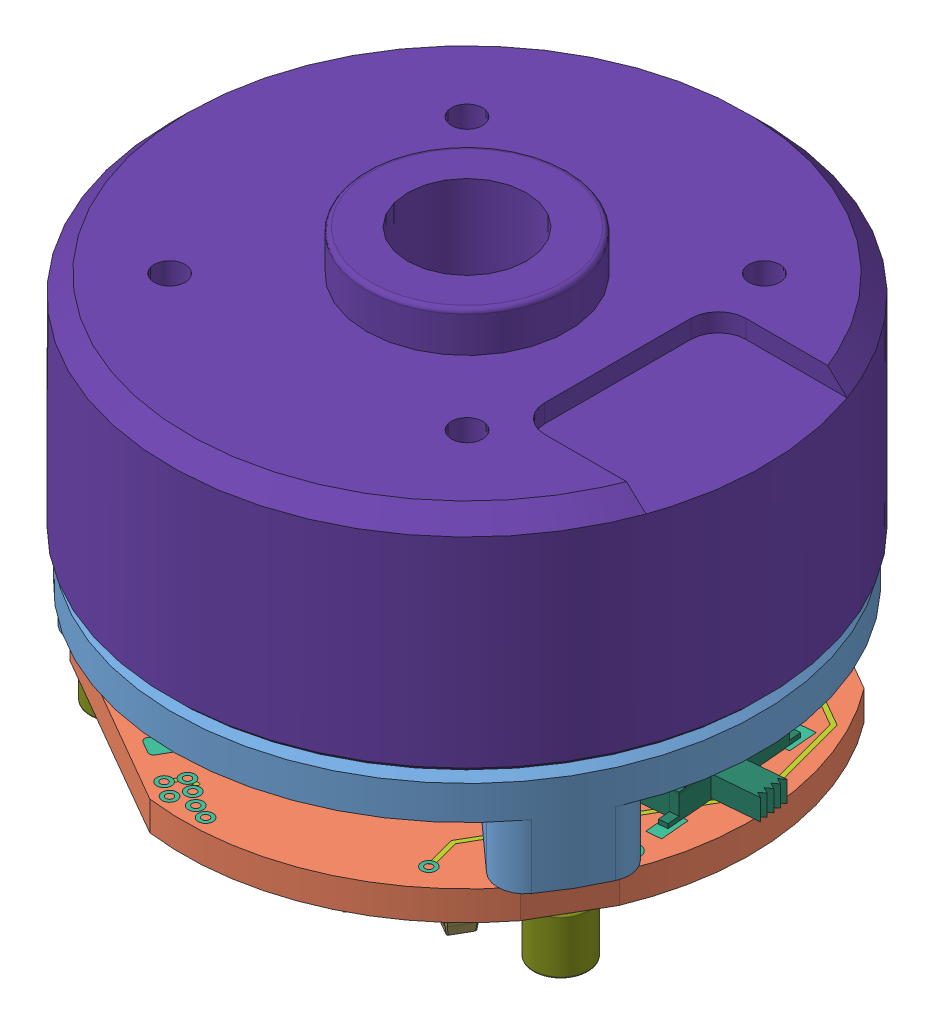
SolidWorks assembly 2804-特价电机 - 孔位修正版-减厚, configuration 默认. Lengths in mm.
Overall size (40.92 25 40.14).
94 component instances, 53 part files, 8 mates.
Components (placement in the parent):
- 复件 零件1^2804-特价电机 - 孔位修正版-减厚-1: 复件 零件1^2804-特价电机 - 孔位修正版-减厚 [默认] x (0 0 -1) z (1 0 0) size (32 6.17 30.88) (virtual)
- S28P12-1: S28P12 [默认] at (0.0001 -7.6 0.0003) x (0.5 0 -0.866025) z (0 -1 0) size (28.6 30.74 6.15)
  - S28P12.step-1: S28P12.step [默认] at origin size (28.6 30.74 6.15)
    - Board_Geoms_db26.step-1: Board_Geoms_db26.step [默认] at origin size (28.6 30.74 1.88)
      - Pcb_db26.step-1: Pcb_db26.step [默认] at (-99.9998 99.9998 0) size (28.6 30.74 1.6)
      - topPads_db26.step-1: topPads_db26.step [默认] at (-99.9998 99.9998 0.02) size (27.56 29.1 0.01)
      - topTracks_db26.step-1: topTracks_db26.step [默认] at (-99.9998 99.9998 0.01) size (26.54 27.25 0.49)
      - topZones_db26.step-1: topZones_db26.step [默认] at (-99.9998 99.9998 0.01) size (16.88 29.66 0.02)
      - botPads_db26.step-1: botPads_db26.step [默认] at (-99.9998 99.9998 -1.62) size (27.7 29.1 0.01)
      - botTracks_db26.step-1: botTracks_db26.step [默认] at (-99.9998 99.9998 -1.61) size (26.06 27.6 0.02)
      - botZones_db26.step-1: botZones_db26.step [默认] at (-99.9998 99.9998 -1.61) size (24.07 13.81 0.01)
    - Step_Models_db26.step-1: Step_Models_db26.step [默认] at origin size (26.96 28.57 6.15)
      - Top_db26.step-1: Top_db26.step [默认] at origin size (24.86 27.45 1.59)
        - U4_PWP059_00006012a0b9.step-1: U4_PWP059_00006012a0b9.step [默认] at (-0.0198 -8.0402 0) x (0 1 0) z (1 0 0) size (6.4 1.2 9.7)
          - PWP28.step-1: PWP28.step [默认] at origin size (1 0.75 0.24)
          - PWP029.step-1: PWP029.step [默认] at origin size (1 0.75 0.24)
          - PWP030.step-1: PWP030.step [默认] at origin size (1 0.75 0.24)
          - PWP031.step-1: PWP031.step [默认] at origin size (1 0.75 0.24)
          - PWP032.step-1: PWP032.step [默认] at origin size (1 0.75 0.24)
          - PWP033.step-1: PWP033.step [默认] at origin size (1 0.75 0.24)
          - PWP034.step-1: PWP034.step [默认] at origin size (1 0.75 0.24)
          - PWP035.step-1: PWP035.step [默认] at origin size (1 0.75 0.24)
          - PWP036.step-1: PWP036.step [默认] at origin size (1 0.75 0.24)
          - PWP037.step-1: PWP037.step [默认] at origin size (1 0.75 0.24)
          - PWP038.step-1: PWP038.step [默认] at origin size (1 0.75 0.24)
          - PWP039.step-1: PWP039.step [默认] at origin size (1 0.75 0.24)
          - PWP040.step-1: PWP040.step [默认] at origin size (1 0.75 0.24)
          - PWP041.step-1: PWP041.step [默认] at origin size (1 0.75 0.24)
          - PWP042.step-1: PWP042.step [默认] at origin size (1 0.75 0.24)
          - PWP043.step-1: PWP043.step [默认] at origin size (1 0.75 0.24)
          - PWP044.step-1: PWP044.step [默认] at origin size (1 0.75 0.24)
          - PWP045.step-1: PWP045.step [默认] at origin size (1 0.75 0.24)
          - PWP046.step-1: PWP046.step [默认] at origin size (1 0.75 0.24)
          - PWP047.step-1: PWP047.step [默认] at origin size (1 0.75 0.24)
          - PWP048.step-1: PWP048.step [默认] at origin size (1 0.75 0.24)
          - PWP049.step-1: PWP049.step [默认] at origin size (1 0.75 0.24)
          - PWP050.step-1: PWP050.step [默认] at origin size (1 0.75 0.24)
          - PWP051.step-1: PWP051.step [默认] at origin size (1 0.75 0.24)
          - PWP052.step-1: PWP052.step [默认] at origin size (1 0.75 0.24)
          - PWP053.step-1: PWP053.step [默认] at origin size (1 0.75 0.24)
          - PWP054.step-1: PWP054.step [默认] at origin size (1 0.75 0.24)
          - PWP055.step-1: PWP055.step [默认] at origin size (1 0.75 0.24)
          - PWP056.step-1: PWP056.step [默认] at origin size (0.55 0.05 0.55)
          - PWP057.step-1: PWP057.step [默认] at origin size (4.4 1.06 9.7)
          - PWP058.step-1: PWP058.step [默认] at origin size (2.75 0.25 5.23)
        - C2_C_0603_1608Metric_00006005682b.step-1: C2_C_0603_1608Metric_00006005682b.step [默认] at (-4.7929 -0.2178 0) x (0 1 0) z (0 0 1) size (1.6 0.8 0.8)
        - C2_C_0603_1608Metric_00006005682b.step-2: C2_C_0603_1608Metric_00006005682b.step [默认] at (-6.2929 -0.2378 0) x (0 1 0) z (0 0 1) size (1.6 0.8 0.8)
        - C2_C_0603_1608Metric_00006005682b.step-3: C2_C_0603_1608Metric_00006005682b.step [默认] at (-5.9698 -10.4127 0) x (0 -1 0) z (0 0 1) size (1.6 0.8 0.8)
        - C2_C_0603_1608Metric_00006005682b.step-4: C2_C_0603_1608Metric_00006005682b.step [默认] at (-9.9829 6.3622 0) x (0 1 0) z (0 0 1) size (1.6 0.8 0.8)
        - C2_C_0603_1608Metric_00006005682b.step-5: C2_C_0603_1608Metric_00006005682b.step [默认] at (7.5102 -10.7002 0) x (0 1 0) z (0 0 1) size (1.6 0.8 0.8)
        - C2_C_0603_1608Metric_00006005682b.step-6: C2_C_0603_1608Metric_00006005682b.step [默认] at (-2.0229 9.3422 0) x (0 1 0) z (0 0 1) size (1.6 0.8 0.8)
        - C2_C_0603_1608Metric_00006005682b.step-7: C2_C_0603_1608Metric_00006005682b.step [默认] at (-5.2298 -13.0102 0) size (1.6 0.8 0.8)
        - C2_C_0603_1608Metric_00006005682b.step-8: C2_C_0603_1608Metric_00006005682b.step [默认] at (-7.4598 -10.4002 0) x (0 1 0) z (0 0 1) size (1.6 0.8 0.8)
        - C2_C_0603_1608Metric_00006005682b.step-9: C2_C_0603_1608Metric_00006005682b.step [默认] at (7.5302 -7.6827 0) x (0 -1 0) z (0 0 1) size (1.6 0.8 0.8)
        - D2_LED_0603_1608Metric_0000600568f0.step-1: D2_LED_0603_1608Metric_0000600568f0.step [默认] at (9.0171 -7.6853 0) x (0 1 0) z (0 0 1) size (1.6 0.8 1.1)
        - R1_R_0603_1608Metric_00006005698f.step-1: R1_R_0603_1608Metric_00006005698f.step [默认] at (10.6096 8.0922 0) x (-1 0 0) z (0 0 1) size (1.6 0.8 0.45)
        - R1_R_0603_1608Metric_00006005698f.step-2: R1_R_0603_1608Metric_00006005698f.step [默认] at (9.2771 -4.0278 0) x (0 1 0) z (0 0 1) size (1.6 0.8 0.45)
        - R1_R_0603_1608Metric_00006005698f.step-3: R1_R_0603_1608Metric_00006005698f.step [默认] at (-3.3129 -1.3653 0) x (0 -1 0) z (0 0 1) size (1.6 0.8 0.45)
        - R1_R_0603_1608Metric_00006005698f.step-4: R1_R_0603_1608Metric_00006005698f.step [默认] at (0.9171 9.3297 0) x (0 1 0) z (0 0 1) size (1.6 0.8 0.45)
        - R1_R_0603_1608Metric_00006005698f.step-5: R1_R_0603_1608Metric_00006005698f.step [默认] at (-1.8229 -1.3653 0) x (0 -1 0) z (0 0 1) size (1.6 0.8 0.45)
        - R1_R_0603_1608Metric_00006005698f.step-6: R1_R_0603_1608Metric_00006005698f.step [默认] at (6.0402 -7.6827 0) x (0 -1 0) z (0 0 1) size (1.6 0.8 0.45)
        - SW1_SW_SPST_B3U-1000P_000060056a0b.step-1: SW1_SW_SPST_B3U-1000P_000060056a0b.step [默认] at (4.6571 9.5022 0) size (4 2.51 1.59)
        - U3_SOT_89_3_000060056a8b.step-1: U3_SOT_89_3_000060056a8b.step [默认] at (-6.7429 8.2822 0) x (0 -1 0) z (0 0 1) size (4 4.5 1.52)
        - C2_C_0603_1608Metric_00006005682b.step-10: C2_C_0603_1608Metric_00006005682b.step [默认] at (10.6096 6.6222 0) x (-1 0 0) z (0 0 1) size (1.6 0.8 0.8)
        - D1_D_0603_00006081285b.step-1: D1_D_0603_00006081285b.step [默认] at (11.3571 1.4022 0) x (0 -1 0) z (0 0 1) size (1.6 0.87 0.66)
        - C2_C_0603_1608Metric_00006005682b.step-11: C2_C_0603_1608Metric_00006005682b.step [默认] at (-6.2729 4.2322 0) x (0 1 0) z (0 0 1) size (1.6 0.8 0.8)
        - C2_C_0603_1608Metric_00006005682b.step-12: C2_C_0603_1608Metric_00006005682b.step [默认] at (7.7671 -4.0153 0) x (0 1 0) z (0 0 1) size (1.6 0.8 0.8)
        - C2_C_0603_1608Metric_00006005682b.step-13: C2_C_0603_1608Metric_00006005682b.step [默认] at (-5.5329 1.9922 0) size (1.6 0.8 0.8)
        - C2_C_0603_1608Metric_00006005682b.step-14: C2_C_0603_1608Metric_00006005682b.step [默认] at (-0.5529 9.3297 0) x (0 -1 0) z (0 0 1) size (1.6 0.8 0.8)
        - C2_C_0603_1608Metric_00006005682b.step-15: C2_C_0603_1608Metric_00006005682b.step [默认] at (11.3571 4.3947 0) x (0 1 0) z (0 0 1) size (1.6 0.8 0.8)
        - C2_C_0603_1608Metric_00006005682b.step-16: C2_C_0603_1608Metric_00006005682b.step [默认] at (-2.5729 0.8622 0) size (1.6 0.8 0.8)
        - R1_R_0603_1608Metric_00006005698f.step-7: R1_R_0603_1608Metric_00006005698f.step [默认] at (-4.8029 4.2097 0) x (0 -1 0) z (0 0 1) size (1.6 0.8 0.45)
        - R1_R_0603_1608Metric_00006005698f.step-8: R1_R_0603_1608Metric_00006005698f.step [默认] at (-5.5529 -2.4578 0) size (1.6 0.8 0.45)
        - U5_LQFP_48_7x7mm_P05mm_000060d40c5b.step-1: U5_LQFP_48_7x7mm_P05mm_000060d40c5b.step [默认] at (5.1427 2.698 0) size (9 9 1.5)
        - R1_R_0603_1608Metric_00006005698f.step-9: R1_R_0603_1608Metric_00006005698f.step [默认] at (6.1396 11.9422 0) x (-1 0 0) z (0 0 1) size (1.6 0.8 0.45)
        - R1_R_0603_1608Metric_00006005698f.step-10: R1_R_0603_1608Metric_00006005698f.step [默认] at (6.1971 -4.0378 0) x (0 1 0) z (0 0 1) size (1.6 0.8 0.45)
        - C2_C_0603_1608Metric_00006005682b.step-17: C2_C_0603_1608Metric_00006005682b.step [默认] at (-9.9829 9.3522 0) x (0 1 0) z (0 0 1) size (1.6 0.8 0.8)
        - C2_C_0603_1608Metric_00006005682b.step-18: C2_C_0603_1608Metric_00006005682b.step [默认] at (-3.4929 9.3497 0) x (0 -1 0) z (0 0 1) size (1.6 0.8 0.8)
        - C2_C_0603_1608Metric_00006005682b.step-19: C2_C_0603_1608Metric_00006005682b.step [默认] at (-7.3579 11.5722 0) size (1.6 0.8 0.8)
        - C22_C_0805_2012Metric_82ecb5eb1270.step-1: C22_C_0805_2012Metric_82ecb5eb1270.step [默认] at (-12.0729 3.8822 0) x (-1 0 0) z (0 0 1) size (2 1.25 1.25)
        - C22_C_0805_2012Metric_82ecb5eb1270.step-2: C22_C_0805_2012Metric_82ecb5eb1270.step [默认] at (-12.0729 1.9122 0) x (-1 0 0) z (0 0 1) size (2 1.25 1.25)
        - C22_C_0805_2012Metric_82ecb5eb1270.step-3: C22_C_0805_2012Metric_82ecb5eb1270.step [默认] at (-12.0629 -4.0078 0) x (-1 0 0) z (0 0 1) size (2 1.25 1.25)
        - C22_C_0805_2012Metric_82ecb5eb1270.step-4: C22_C_0805_2012Metric_82ecb5eb1270.step [默认] at (-12.0729 -0.0578 0) x (-1 0 0) z (0 0 1) size (2 1.25 1.25)
        - VR1_SOT_23_081ca162a7f8.step-1: VR1_SOT_23_081ca162a7f8.step [默认] at (-3.9429 12.5422 0) x (-1 0 0) z (0 0 1) size (2.5 3 1.2)
        - C2_C_0603_1608Metric_00006005682b.step-20: C2_C_0603_1608Metric_00006005682b.step [默认] at (3.1571 11.9522 0) x (-1 0 0) z (0 0 1) size (1.6 0.8 0.8)
        - C22_C_0805_2012Metric_82ecb5eb1270.step-5: C22_C_0805_2012Metric_82ecb5eb1270.step [默认] at (-12.0629 -2.0378 0) x (-1 0 0) z (0 0 1) size (2 1.25 1.25)
      - Bot_db26.step-1: Bot_db26.step [默认] at origin size (16.88 18.18 3.54)
        - J4_SM04B-SRSS_000060d40966[2].step-1: J4_SM04B-SRSS_000060d40966[2].step [默认] at (9.988 -0.0178 -1.3) x (0 -1 0) z (1 0 0) size (6 2.96 4.95)
        - U2_SOIC_8_39x49mm_P127mm_000060d5d58d.step-1: U2_SOIC_8_39x49mm_P127mm_000060d5d58d.step [默认] at (0.0002 -0.0002 -1.6) x (1 0 0) z (0 0 -1) size (6 4.9 1.75)
        - SW2_Selector Switch - MSK1103_000061156a95.step-1: SW2_Selector Switch - MSK1103_000061156a95.step [默认] at (2.8725 14.2724 -1.6) x (0.819152 -0.573576 0) z (0.573576 0.819152 0) size (7.98 2.01 6.19)
- 复件 零件19^2804-特价电机 - 孔位修正版-减厚-1: 复件 零件19^2804-特价电机 - 孔位修正版-减厚 [默认] at (-12.1244 -10.6 7) x (0.999963 0 0.008553) z (-0.008553 0 0.999963) size (3 3 3) (virtual)
- 复件 零件75^2804-特价电机 - 孔位修正版-减厚-1: 复件 零件75^2804-特价电机 - 孔位修正版-减厚 [默认] at origin size (32.5 18 32.5) (virtual)
- 复件 零件19^2804-特价电机 - 孔位修正版-减厚-2: 复件 零件19^2804-特价电机 - 孔位修正版-减厚 [默认] at (0 -10.6 -14) x (-0.507389 0 0.861717) z (-0.861717 0 -0.507389) size (3 3 3) (virtual)
- 复件 零件19^2804-特价电机 - 孔位修正版-减厚-3: 复件 零件19^2804-特价电机 - 孔位修正版-减厚 [默认] at (12.1244 -10.6 7) x (-0.492575 0 -0.87027) z (0.87027 0 -0.492575) size (3 3 3) (virtual)
Mates (geometry in assembly coordinates):
- 重合1: coincident anti-aligned: plane of 电机-1 through (0 0 0) normal (0 -1 0); plane of 复件 零件1^装配体1_2805特价电机-2轴-1 through (0 0 0) normal (0 1 0)
- 同心1: concentric aligned: cylinder of 电机-1 through (11.5 5 0) axis (0 -1 0) radius 0.85; cylinder of 复件 零件1^装配体1_2805特价电机-2轴-1 through (11.5 0 0) axis (0 -1 0) radius 1.1
- 同心2: concentric anti-aligned: cylinder of 电机-1 through (0 12.2 0) axis (0 -1 0) radius 16.25; cylinder of 复件 零件1^装配体1_2805特价电机-2轴-1 through (0 -6 0) axis (0 1 0) radius 16
- 重合2: coincident anti-aligned: plane of 复件 零件1^装配体1_2805特价电机-2轴-1 through (0 -6 0) normal (0 -1 0); plane of S28P12-1/S28P12.step-1/Board_Geoms_db26.step-1/Pcb_db26.step-1 through (0.0001 -6 0.0002) normal (0 1 0)
- 同心4: concentric anti-aligned: cylinder of 复件 零件1^装配体1_2805特价电机-2轴-1 through (0 -6 -14) axis (0 1 0) radius 0.925; cylinder of S28P12-1/S28P12.step-1/Board_Geoms_db26.step-1/Pcb_db26.step-1 through (0 -7.6 -14) axis (0 -1 0) radius 1.1
- 同心3: concentric aligned: cylinder of 电机-1 through (0 12.2 0) axis (0 -1 0) radius 16.25; cylinder of S28P12-1/S28P12.step-1/Board_Geoms_db26.step-1/Pcb_db26.step-1 through (0 -7.6 0) axis (0 -1 0) radius 15.4963
- 重合3: coincident anti-aligned: plane of S28P12-1/S28P12.step-1/Board_Geoms_db26.step-1/Pcb_db26.step-1 through (0.0001 -7.6 0.0002) normal (0 -1 0); plane of 铜柱-1 through (-12.1244 -7.6 7) normal (0 1 0)
- 同心5: concentric aligned: cylinder of S28P12-1/S28P12.step-1/Board_Geoms_db26.step-1/Pcb_db26.step-1 through (-12.1244 -7.6 7) axis (0 -1 0) radius 1.1; cylinder of 铜柱-1 through (-12.1244 -7.6 7) axis (0 -1 0) radius 1.5
